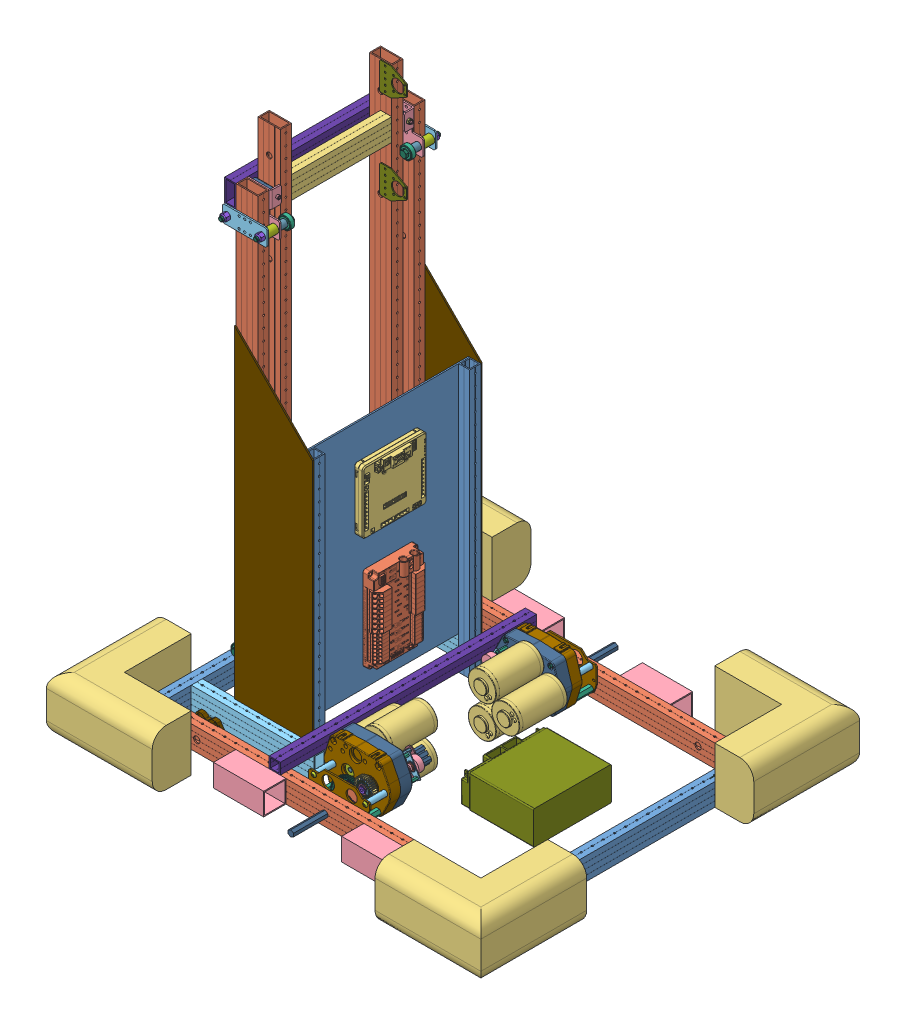
SolidWorks assembly Test Robot 3, configuration Default. Lengths in mm. (continued)
Components (placement in the parent): (continued)
- Test Base 3-1: Test Base 3 [Default] at (-213.2986 -131.6714 217.4582) size (990.6 641.86 863.6) (continued)
  - 3 CIM Ball Shifter with WCD Output-2: 3 CIM Ball Shifter with WCD Output [Default] at (640.2827 400.7203 338.8075) x (0 1 0) z (0 0 -1) size (169.11 183.68 312.65) (continued)
    - 217-3288-001 Rev3-1: 217-3288-001 Rev3 [Default] at (0 0 0.0889) x (0.055929 -0.998435 0) z (0 0 1) size (99.51 99.53 98.3) (continued)
      - 217-2428-007 Rev1-4: 217-2428-007 Rev1 [Default] at (0 -6.275 26.9494) x (-0.766153 0.629782 0.128005) z (-0.605376 -0.640389 -0.472676) size (6.35 6.35 6.35)
      - 217-2428-007 Rev1-5: 217-2428-007 Rev1 [Default] at (-7.809 4.5085 14.2494) x (-0.049287 -0.826019 -0.561483) z (0.929754 -0.24331 0.276329) size (6.35 6.35 6.35)
      - 217-2428-007 Rev1-6: 217-2428-007 Rev1 [Default] at (0 -9.017 14.2494) x (0.739997 0.370326 -0.561483) z (-0.254164 0.926846 0.276329) size (6.35 6.35 6.35)
    - 217-3210-001 Rev1_30t-1: 217-3210-001 Rev1_30t [Default] at (0 53.4162 30.0736) x (-0.966828 0.255427 0) z (0 0 1) size (41.01 41.12 12.65)
    - 217-2711-002 Rev1_50t-1: 217-2711-002 Rev1_50t [Default] at (0 53.4162 17.4244) x (0.262208 -0.965011 0) z (0 0 1) size (66.7 66.76 12.65)
  - Base Front Rail-2: Base Front Rail [Default] at (1069.5219 360.9185 -429.2377) size (25.4 50.8 152.4)
  - Blue Bumper-3: Blue Bumper [Default] at (180.5219 335.5185 942.3623) size (241.3 127 241.3)
  - Blue Bumper-4: Blue Bumper [Default] at (180.5219 335.5185 78.7623) x (0 0 1) z (-1 0 0) size (241.3 127 241.3)
  - Battery_12V-1: Battery_12V [Default] at (955.2219 397.7318 461.8714) x (0 0 1) z (-1 0 0) size (177.8 76.2 167.13)
  - Superstructure Lower Crossbar-2: Superstructure Lower Crossbar [Default] at (561.5219 399.0185 967.7623) x (0 1 0) z (0 0 -1) size (25.4 25.4 584.2)
  - Base Rear Rail-2: Base Rear Rail [Default] at (1069.5219 360.9185 104.1623) size (25.4 50.8 685.8)
  - 217-3432-STEP-v2-1: 217-3432-STEP-v2 [Default] at (383.7219 362.5822 245.4498) size (69.4 66.32 9.53)
  - 217-3432-STEP-v2-2: 217-3432-STEP-v2 [Default] at (383.7219 362.5822 775.6748) x (-1 0 0) z (0 0 -1) size (69.4 66.32 9.53)
  - Electronics Upright-1: Electronics Upright [Default] at (536.1219 1084.8185 688.3623) x (1 0 0) z (0 -1 0) size (25.4 25.4 609.6)
  - Electronics Upright-2: Electronics Upright [Default] at (536.1219 1084.8185 332.7623) x (1 0 0) z (0 -1 0) size (25.4 25.4 609.6)
- Elevator Moving Stage-1: Elevator Moving Stage [Default] at (-744.0684 626.0553 1293.6415) x (0 0 -1) z (1 0 0) size (355.24 1067.72 119.92)
  - Elevator Fixed Frame-1: Elevator Fixed Frame [Default] at (692.621 1.7594 927.1918) x (1 0 0) z (0 1 0) size (25.4 50.8 1066.8)
  - Elevator Fixed Frame-2: Elevator Fixed Frame [Default] at (438.621 1.7594 927.1918) x (1 0 0) z (0 1 0) size (25.4 50.8 1066.8)
  - Elevator Crossbar-1: Elevator Crossbar [Default] at (1200.621 -252.2406 927.1918) x (0 -1 0) z (-1 0 0) size (25.4 50.8 228.6)
  - am-3844+2x1+Elevator+Assembly+Example-1: am-3844+2x1+Elevator+Assembly+Example [Default] at (298.921 81.9689 954.3698) x (-1 0 0) z (0 0 1) size (82.37 89.82 113.91)
    - Example Single Corner Bearing Assembly-1: Example Single Corner Bearing Assembly [Default] at (-442.3285 289.2703 9.4128) x (0 0 1) z (-1 0 0) size (113.91 89.82 82.37)
      - Large Bearing Block Plate-1: Large Bearing Block Plate [Default] at (-85.6128 70.3392 -35.9285) x (1 0 0) z (0 -1 0) size (101.6 24.99 88.9)
      - Small Bearing Block Plate-1: Small Bearing Block Plate [Default] at (-85.6128 70.3392 -64.5035) x (1 0 0) z (0 -1 0) size (101.6 3.17 38.1)
      - 1614Z Bearing-1: 1614Z Bearing [Default] at (-74.6273 89.3892 -8.941) x (-0.590982 0.806685 0) z (0 0 1) size (28.58 28.58 9.53)
      - 1614Z Bearing-2: 1614Z Bearing [Default] at (5.0017 89.3892 -8.941) x (0.001674 0.999999 0) z (0 0 1) size (28.58 28.58 9.53)
      - AS75-18-64 Aluminum Spacer-1: AS75-18-64 Aluminum Spacer [Default] at (5.0017 89.3892 -35.9285) x (-0.668699 0.743533 0) z (-0.743533 -0.668699 0) size (19.05 25.41 19.05)
      - AS75-18-64 Aluminum Spacer-2: AS75-18-64 Aluminum Spacer [Default] at (-74.6273 89.3892 -61.3285) x (0.536222 0.844077 0) z (0.844077 -0.536222 0) size (19.05 25.41 19.05)
      - 3-8-16 NyLock Nut - Mcm 95615A140_95615A140-1: 3-8-16 NyLock Nut - Mcm 95615A140_95615A140 [Default] at (5.0017 89.3892 -64.5035) x (1 0 0) z (0 1 0) size (14.29 12 16.5)
      - 3-8-16 NyLock Nut - Mcm 95615A140_95615A140-2: 3-8-16 NyLock Nut - Mcm 95615A140_95615A140 [Default] at (-74.6273 89.3892 -64.5035) x (1 0 0) z (0 1 0) size (14.29 12 16.5)
      - am-0602 .250 x .192 x 2.14 Brass Tube-1: am-0602 .250 x .192 x 2.14 Brass Tube [Default] at (-7.6348 38.5892 -20.4599) x (0 0 1) z (-1 0 0) size (6.35 6.35 54.36)
      - 13RS075051 .750 x .260 x 1.00 Spacer-1: 13RS075051 .750 x .260 x 1.00 Spacer [Default] at (-60.2128 38.5892 -20.4599) x (0 -0.722855 0.691) z (0 0.691 0.722855) size (19.05 25.4 19.05)
      - 13RS075051 .750 x .260 x 1.00 Spacer-2: 13RS075051 .750 x .260 x 1.00 Spacer [Default] at (-34.8128 38.5892 -20.4599) x (0 -0.801304 -0.598258) z (0 -0.598258 0.801304) size (19.05 25.4 19.05)
      - 0.25 Flat Washer_Preferred Wide FW 0.25-1: 0.25 Flat Washer_Preferred Wide FW 0.25 [Default] at (-60.2128 38.5892 -20.4599) x (1 0 0) z (0 -0.116572 0.993182) size (1.4 15.88 15.88)
      - 0.25 Flat Washer_Preferred Wide FW 0.25-2: 0.25 Flat Washer_Preferred Wide FW 0.25 [Default] at (-8.0158 38.5892 -20.4599) size (1.4 15.88 15.88)
      - 10-32 Nylock Nut-1: 10-32 Nylock Nut [Default] at (-65.1658 38.5892 -20.4599) x (0 -0.097883 0.995198) z (-1 0 0) size (9.53 11 5.96)
      - SHCS 10-32 x 2.75_HX-SHCS 0.19-32x2.75x0.875-C-1: SHCS 10-32 x 2.75_HX-SHCS 0.19-32x2.75x0.875-C [Default] at (0.3662 38.5892 -20.4599) x (-1 0 0) z (0 0.982583 -0.185827) size (74.68 7.94 7.94)
      - AS62-18-56 Aluminum Spacer-1: AS62-18-56 Aluminum Spacer [Default] at (5.0017 89.3892 -13.7035) x (0.977193 0.212353 0) z (-0.212353 0.977193 0) size (15.88 19.06 15.88)
      - AS62-18-56 Aluminum Spacer-2: AS62-18-56 Aluminum Spacer [Default] at (-74.6273 89.3892 -13.7035) x (1 0 0) z (0 1 0) size (15.88 19.06 15.88)
      - 375-16 x 3 Hex Bolt_HFBOLT 0.375-16x2.5x1-C-1: 375-16 x 3 Hex Bolt_HFBOLT 0.375-16x2.5x1-C [Default] at (-74.6273 89.3892 1.9937) x (0 0 -1) z (1 0 0) size (82.37 16.48 14.28)
      - 375-16 x 3 Hex Bolt_HFBOLT 0.375-16x2.5x1-C-2: 375-16 x 3 Hex Bolt_HFBOLT 0.375-16x2.5x1-C [Default] at (5.0017 89.3892 1.9937) x (0 0 -1) z (-0.5 -0.866025 0) size (82.37 16.48 14.28)
  - am-3844+2x1+Elevator+Assembly+Example-2: am-3844+2x1+Elevator+Assembly+Example [Default] at (832.321 81.9689 900.0138) x (1 0 0) z (0 0 -1) size (82.37 89.82 113.91)
    - Example Single Corner Bearing Assembly-1: Example Single Corner Bearing Assembly [Default] at (-442.3285 289.2703 9.4128) x (0 0 1) z (-1 0 0) size (113.91 89.82 82.37)
      - Large Bearing Block Plate-1: Large Bearing Block Plate [Default] at (-85.6128 70.3392 -35.9285) x (1 0 0) z (0 -1 0) size (101.6 24.99 88.9)
      - Small Bearing Block Plate-1: Small Bearing Block Plate [Default] at (-85.6128 70.3392 -64.5035) x (1 0 0) z (0 -1 0) size (101.6 3.17 38.1)
      - 1614Z Bearing-1: 1614Z Bearing [Default] at (-74.6273 89.3892 -8.941) x (-0.590982 0.806685 0) z (0 0 1) size (28.58 28.58 9.53)
      - 1614Z Bearing-2: 1614Z Bearing [Default] at (5.0017 89.3892 -8.941) x (0.001674 0.999999 0) z (0 0 1) size (28.58 28.58 9.53)
      - AS75-18-64 Aluminum Spacer-1: AS75-18-64 Aluminum Spacer [Default] at (5.0017 89.3892 -35.9285) x (-0.668699 0.743533 0) z (-0.743533 -0.668699 0) size (19.05 25.41 19.05)
      - AS75-18-64 Aluminum Spacer-2: AS75-18-64 Aluminum Spacer [Default] at (-74.6273 89.3892 -61.3285) x (0.536222 0.844077 0) z (0.844077 -0.536222 0) size (19.05 25.41 19.05)
      - 3-8-16 NyLock Nut - Mcm 95615A140_95615A140-1: 3-8-16 NyLock Nut - Mcm 95615A140_95615A140 [Default] at (5.0017 89.3892 -64.5035) x (1 0 0) z (0 1 0) size (14.29 12 16.5)
      - 3-8-16 NyLock Nut - Mcm 95615A140_95615A140-2: 3-8-16 NyLock Nut - Mcm 95615A140_95615A140 [Default] at (-74.6273 89.3892 -64.5035) x (1 0 0) z (0 1 0) size (14.29 12 16.5)
      - am-0602 .250 x .192 x 2.14 Brass Tube-1: am-0602 .250 x .192 x 2.14 Brass Tube [Default] at (-7.6348 38.5892 -20.4599) x (0 0 1) z (-1 0 0) size (6.35 6.35 54.36)
      - 13RS075051 .750 x .260 x 1.00 Spacer-1: 13RS075051 .750 x .260 x 1.00 Spacer [Default] at (-60.2128 38.5892 -20.4599) x (0 -0.722855 0.691) z (0 0.691 0.722855) size (19.05 25.4 19.05)
      - 13RS075051 .750 x .260 x 1.00 Spacer-2: 13RS075051 .750 x .260 x 1.00 Spacer [Default] at (-34.8128 38.5892 -20.4599) x (0 -0.801304 -0.598258) z (0 -0.598258 0.801304) size (19.05 25.4 19.05)
      - 0.25 Flat Washer_Preferred Wide FW 0.25-1: 0.25 Flat Washer_Preferred Wide FW 0.25 [Default] at (-60.2128 38.5892 -20.4599) x (1 0 0) z (0 -0.116572 0.993182) size (1.4 15.88 15.88)
      - 0.25 Flat Washer_Preferred Wide FW 0.25-2: 0.25 Flat Washer_Preferred Wide FW 0.25 [Default] at (-8.0158 38.5892 -20.4599) size (1.4 15.88 15.88)
      - 10-32 Nylock Nut-1: 10-32 Nylock Nut [Default] at (-65.1658 38.5892 -20.4599) x (0 -0.097883 0.995198) z (-1 0 0) size (9.53 11 5.96)
      - SHCS 10-32 x 2.75_HX-SHCS 0.19-32x2.75x0.875-C-1: SHCS 10-32 x 2.75_HX-SHCS 0.19-32x2.75x0.875-C [Default] at (0.3662 38.5892 -20.4599) x (-1 0 0) z (0 0.982583 -0.185827) size (74.68 7.94 7.94)
      - AS62-18-56 Aluminum Spacer-1: AS62-18-56 Aluminum Spacer [Default] at (5.0017 89.3892 -13.7035) x (0.977193 0.212353 0) z (-0.212353 0.977193 0) size (15.88 19.06 15.88)
      - AS62-18-56 Aluminum Spacer-2: AS62-18-56 Aluminum Spacer [Default] at (-74.6273 89.3892 -13.7035) x (1 0 0) z (0 1 0) size (15.88 19.06 15.88)
      - 375-16 x 3 Hex Bolt_HFBOLT 0.375-16x2.5x1-C-1: 375-16 x 3 Hex Bolt_HFBOLT 0.375-16x2.5x1-C [Default] at (-74.6273 89.3892 1.9937) x (0 0 -1) z (1 0 0) size (82.37 16.48 14.28)
      - 375-16 x 3 Hex Bolt_HFBOLT 0.375-16x2.5x1-C-2: 375-16 x 3 Hex Bolt_HFBOLT 0.375-16x2.5x1-C [Default] at (5.0017 89.3892 1.9937) x (0 0 -1) z (-0.5 -0.866025 0) size (82.37 16.48 14.28)
  - VersaFrame Side Bearing Mount-1: VersaFrame Side Bearing Mount [Default] at (677.635 719.3094 968.4668) x (0 -1 0) z (1 0 0) size (63.5 61.91 2.29)
  - Elevator Crossbar-2: Elevator Crossbar [Default] at (-69.379 624.0594 939.8918) x (0 0 -1) z (1 0 0) size (25.4 50.8 228.6)
  - VersaFrame Side Bearing Mount-2: VersaFrame Side Bearing Mount [Default] at (677.635 516.1094 968.4668) x (0 -1 0) z (1 0 0) size (63.5 61.91 2.29)
- Elevator Base Frame-1: Elevator Base Frame [Default] at (917.7191 512.449 119.177) x (0 0 1) z (-1 0 0) size (419.1 1066.8 119.57)
  - Elevator Fixed Frame-1: Elevator Fixed Frame [Default] at (786.6435 8.8982 734.5957) x (1 0 0) z (0 1 0) size (25.4 50.8 1066.8)
  - Elevator Fixed Frame-2: Elevator Fixed Frame [Default] at (431.0435 8.8982 734.5957) x (1 0 0) z (0 1 0) size (25.4 50.8 1066.8)
  - am-3844+2x1+Elevator+Assembly+Example-1: am-3844+2x1+Elevator+Assembly+Example [Default] at (37.3435 1067.0077 761.7737) x (-1 0 0) z (0 0 1) size (82.37 89.82 113.91)
    - Example Single Corner Bearing Assembly-1: Example Single Corner Bearing Assembly [Default] at (-442.3285 289.2703 9.4128) x (0 0 1) z (-1 0 0) size (113.91 89.82 82.37)
      - Large Bearing Block Plate-1: Large Bearing Block Plate [Default] at (-85.6128 70.3392 -35.9285) x (1 0 0) z (0 -1 0) size (101.6 24.99 88.9)
      - Small Bearing Block Plate-1: Small Bearing Block Plate [Default] at (-85.6128 70.3392 -64.5035) x (1 0 0) z (0 -1 0) size (101.6 3.17 38.1)
      - 1614Z Bearing-1: 1614Z Bearing [Default] at (-74.6273 89.3892 -8.941) x (-0.590982 0.806685 0) z (0 0 1) size (28.58 28.58 9.53)
      - 1614Z Bearing-2: 1614Z Bearing [Default] at (5.0017 89.3892 -8.941) x (0.001674 0.999999 0) z (0 0 1) size (28.58 28.58 9.53)
      - AS75-18-64 Aluminum Spacer-1: AS75-18-64 Aluminum Spacer [Default] at (5.0017 89.3892 -35.9285) x (-0.668699 0.743533 0) z (-0.743533 -0.668699 0) size (19.05 25.41 19.05)
      - AS75-18-64 Aluminum Spacer-2: AS75-18-64 Aluminum Spacer [Default] at (-74.6273 89.3892 -61.3285) x (0.536222 0.844077 0) z (0.844077 -0.536222 0) size (19.05 25.41 19.05)
      - 3-8-16 NyLock Nut - Mcm 95615A140_95615A140-1: 3-8-16 NyLock Nut - Mcm 95615A140_95615A140 [Default] at (5.0017 89.3892 -64.5035) x (1 0 0) z (0 1 0) size (14.29 12 16.5)
      - 3-8-16 NyLock Nut - Mcm 95615A140_95615A140-2: 3-8-16 NyLock Nut - Mcm 95615A140_95615A140 [Default] at (-74.6273 89.3892 -64.5035) x (1 0 0) z (0 1 0) size (14.29 12 16.5)
      - am-0602 .250 x .192 x 2.14 Brass Tube-1: am-0602 .250 x .192 x 2.14 Brass Tube [Default] at (-7.6348 38.5892 -20.4599) x (0 0 1) z (-1 0 0) size (6.35 6.35 54.36)
      - 13RS075051 .750 x .260 x 1.00 Spacer-1: 13RS075051 .750 x .260 x 1.00 Spacer [Default] at (-60.2128 38.5892 -20.4599) x (0 -0.722855 0.691) z (0 0.691 0.722855) size (19.05 25.4 19.05)
      - 13RS075051 .750 x .260 x 1.00 Spacer-2: 13RS075051 .750 x .260 x 1.00 Spacer [Default] at (-34.8128 38.5892 -20.4599) x (0 -0.801304 -0.598258) z (0 -0.598258 0.801304) size (19.05 25.4 19.05)
      - 0.25 Flat Washer_Preferred Wide FW 0.25-1: 0.25 Flat Washer_Preferred Wide FW 0.25 [Default] at (-60.2128 38.5892 -20.4599) x (1 0 0) z (0 -0.116572 0.993182) size (1.4 15.88 15.88)
      - 0.25 Flat Washer_Preferred Wide FW 0.25-2: 0.25 Flat Washer_Preferred Wide FW 0.25 [Default] at (-8.0158 38.5892 -20.4599) size (1.4 15.88 15.88)
      - 10-32 Nylock Nut-1: 10-32 Nylock Nut [Default] at (-65.1658 38.5892 -20.4599) x (0 -0.097883 0.995198) z (-1 0 0) size (9.53 11 5.96)
      - SHCS 10-32 x 2.75_HX-SHCS 0.19-32x2.75x0.875-C-1: SHCS 10-32 x 2.75_HX-SHCS 0.19-32x2.75x0.875-C [Default] at (0.3662 38.5892 -20.4599) x (-1 0 0) z (0 0.982583 -0.185827) size (74.68 7.94 7.94)
      - AS62-18-56 Aluminum Spacer-1: AS62-18-56 Aluminum Spacer [Default] at (5.0017 89.3892 -13.7035) x (0.977193 0.212353 0) z (-0.212353 0.977193 0) size (15.88 19.06 15.88)
      - AS62-18-56 Aluminum Spacer-2: AS62-18-56 Aluminum Spacer [Default] at (-74.6273 89.3892 -13.7035) x (1 0 0) z (0 1 0) size (15.88 19.06 15.88)
      - 375-16 x 3 Hex Bolt_HFBOLT 0.375-16x2.5x1-C-1: 375-16 x 3 Hex Bolt_HFBOLT 0.375-16x2.5x1-C [Default] at (-74.6273 89.3892 1.9937) x (0 0 -1) z (1 0 0) size (82.37 16.48 14.28)
      - 375-16 x 3 Hex Bolt_HFBOLT 0.375-16x2.5x1-C-2: 375-16 x 3 Hex Bolt_HFBOLT 0.375-16x2.5x1-C [Default] at (5.0017 89.3892 1.9937) x (0 0 -1) z (-0.5 -0.866025 0) size (82.37 16.48 14.28)
  - am-3844+2x1+Elevator+Assembly+Example-2: am-3844+2x1+Elevator+Assembly+Example [Default] at (1180.3435 1067.0077 710.9737) x (1 0 0) z (0 0 -1) size (82.37 89.82 113.91)
    - Example Single Corner Bearing Assembly-1: Example Single Corner Bearing Assembly [Default] at (-442.3285 289.2703 9.4128) x (0 0 1) z (-1 0 0) size (113.91 89.82 82.37)
      - Large Bearing Block Plate-1: Large Bearing Block Plate [Default] at (-85.6128 70.3392 -35.9285) x (1 0 0) z (0 -1 0) size (101.6 24.99 88.9)
      - Small Bearing Block Plate-1: Small Bearing Block Plate [Default] at (-85.6128 70.3392 -64.5035) x (1 0 0) z (0 -1 0) size (101.6 3.17 38.1)
      - 1614Z Bearing-1: 1614Z Bearing [Default] at (-74.6273 89.3892 -8.941) x (-0.590982 0.806685 0) z (0 0 1) size (28.58 28.58 9.53)
      - 1614Z Bearing-2: 1614Z Bearing [Default] at (5.0017 89.3892 -8.941) x (0.001674 0.999999 0) z (0 0 1) size (28.58 28.58 9.53)
      - AS75-18-64 Aluminum Spacer-1: AS75-18-64 Aluminum Spacer [Default] at (5.0017 89.3892 -35.9285) x (-0.668699 0.743533 0) z (-0.743533 -0.668699 0) size (19.05 25.41 19.05)
      - AS75-18-64 Aluminum Spacer-2: AS75-18-64 Aluminum Spacer [Default] at (-74.6273 89.3892 -61.3285) x (0.536222 0.844077 0) z (0.844077 -0.536222 0) size (19.05 25.41 19.05)
      - 3-8-16 NyLock Nut - Mcm 95615A140_95615A140-1: 3-8-16 NyLock Nut - Mcm 95615A140_95615A140 [Default] at (5.0017 89.3892 -64.5035) x (1 0 0) z (0 1 0) size (14.29 12 16.5)
      - 3-8-16 NyLock Nut - Mcm 95615A140_95615A140-2: 3-8-16 NyLock Nut - Mcm 95615A140_95615A140 [Default] at (-74.6273 89.3892 -64.5035) x (1 0 0) z (0 1 0) size (14.29 12 16.5)
      - am-0602 .250 x .192 x 2.14 Brass Tube-1: am-0602 .250 x .192 x 2.14 Brass Tube [Default] at (-7.6348 38.5892 -20.4599) x (0 0 1) z (-1 0 0) size (6.35 6.35 54.36)
      - 13RS075051 .750 x .260 x 1.00 Spacer-1: 13RS075051 .750 x .260 x 1.00 Spacer [Default] at (-60.2128 38.5892 -20.4599) x (0 -0.722855 0.691) z (0 0.691 0.722855) size (19.05 25.4 19.05)
      - 13RS075051 .750 x .260 x 1.00 Spacer-2: 13RS075051 .750 x .260 x 1.00 Spacer [Default] at (-34.8128 38.5892 -20.4599) x (0 -0.801304 -0.598258) z (0 -0.598258 0.801304) size (19.05 25.4 19.05)
      - 0.25 Flat Washer_Preferred Wide FW 0.25-1: 0.25 Flat Washer_Preferred Wide FW 0.25 [Default] at (-60.2128 38.5892 -20.4599) x (1 0 0) z (0 -0.116572 0.993182) size (1.4 15.88 15.88)
      - 0.25 Flat Washer_Preferred Wide FW 0.25-2: 0.25 Flat Washer_Preferred Wide FW 0.25 [Default] at (-8.0158 38.5892 -20.4599) size (1.4 15.88 15.88)
      - 10-32 Nylock Nut-1: 10-32 Nylock Nut [Default] at (-65.1658 38.5892 -20.4599) x (0 -0.097883 0.995198) z (-1 0 0) size (9.53 11 5.96)
      - SHCS 10-32 x 2.75_HX-SHCS 0.19-32x2.75x0.875-C-1: SHCS 10-32 x 2.75_HX-SHCS 0.19-32x2.75x0.875-C [Default] at (0.3662 38.5892 -20.4599) x (-1 0 0) z (0 0.982583 -0.185827) size (74.68 7.94 7.94)
      - AS62-18-56 Aluminum Spacer-1: AS62-18-56 Aluminum Spacer [Default] at (5.0017 89.3892 -13.7035) x (0.977193 0.212353 0) z (-0.212353 0.977193 0) size (15.88 19.06 15.88)
      - AS62-18-56 Aluminum Spacer-2: AS62-18-56 Aluminum Spacer [Default] at (-74.6273 89.3892 -13.7035) x (1 0 0) z (0 1 0) size (15.88 19.06 15.88)
      - 375-16 x 3 Hex Bolt_HFBOLT 0.375-16x2.5x1-C-1: 375-16 x 3 Hex Bolt_HFBOLT 0.375-16x2.5x1-C [Default] at (-74.6273 89.3892 1.9937) x (0 0 -1) z (1 0 0) size (82.37 16.48 14.28)
      - 375-16 x 3 Hex Bolt_HFBOLT 0.375-16x2.5x1-C-2: 375-16 x 3 Hex Bolt_HFBOLT 0.375-16x2.5x1-C [Default] at (5.0017 89.3892 1.9937) x (0 0 -1) z (-0.5 -0.866025 0) size (82.37 16.48 14.28)
  - Frame Crossbar-1: Frame Crossbar [Default] at (1167.6435 732.7982 772.6957) x (0 0 1) z (-1 0 0) size (25.4 50.8 381)
- Elevator Side Panels-1: Elevator Side Panels [Default] at (157.7234 254.6472 918.5205) size (177.8 736.6 3.17)
- Elevator Side Panels-2: Elevator Side Panels [Default] at (157.7234 254.6472 534.3455) size (177.8 736.6 3.17)
- Electronics Panel-1: Electronics Panel [Default] at (306.9484 280.0472 918.5205) x (0 0 -1) z (1 0 0) size (381 533.4 3.17)
- PowerDistributionPanel-1: PowerDistributionPanel [Default] at (316.8036 414.5094 723.415) x (0 -1 0) z (0 0 1) size (192.68 39.24 124.89)
- roboRIO-1: roboRIO [Default] at (319.7754 665.6573 728.661) x (0 0 -1) z (1 0 0) size (146.27 143.19 36.83)
Mates (geometry in assembly coordinates):
- Coincident1: coincident anti-aligned: plane of Test Base 3-1/Base Side Rail Internal-1 through (360.9234 203.8472 918.5205) normal (0 0 -1); plane of Elevator Base Frame-1/Elevator Fixed Frame-1 through (157.7234 1270.6472 918.5205) normal (0 0 1)
- Coincident2: coincident aligned: plane of Test Base 3-1/Base Side Rail Internal-1 through (360.9234 203.8472 943.9205) normal (0 -1 0); plane of Elevator Base Frame-1/Elevator Fixed Frame-1 through (183.1234 203.8472 905.8205) normal (0 -1 0)
- Distance1: distance = 76.2 mm anti-aligned: plane of Elevator Base Frame-1/Elevator Fixed Frame-1 through (157.7234 1270.6472 893.1205) normal (-1 0 0); plane of Test Base 3-1/Base Rear Rail-1 through (81.5234 203.8472 1070.9205) normal (1 0 0)
- Coincident3: coincident aligned: plane of Elevator Moving Stage-1/Elevator Fixed Frame-1 through (208.5234 1377.1147 613.7205) normal (1 0 0); plane of Elevator Base Frame-1/Elevator Fixed Frame-2 through (208.5234 1270.6472 537.5205) normal (1 0 0)
- Distance2: distance = 25.4 mm anti-aligned: plane of Elevator Moving Stage-1/Elevator Fixed Frame-1 through (208.5234 1377.1147 588.3205) normal (0 0 -1); plane of Elevator Base Frame-1/Elevator Fixed Frame-2 through (157.7234 1270.6472 562.9205) normal (0 0 1)
- Coincident4: coincident anti-aligned: plane of Elevator Base Frame-1/Elevator Fixed Frame-1 through (157.7234 1270.6472 918.5205) normal (0 0 1); plane of Elevator Side Panels-1 through (157.7234 254.6472 918.5205) normal (0 0 -1)
- Coincident5: coincident aligned: plane of Elevator Base Frame-1/Elevator Fixed Frame-1 through (157.7234 1270.6472 893.1205) normal (-1 0 0); plane of Elevator Side Panels-1 through (157.7234 254.6472 921.6955) normal (-1 0 0)
- Coincident7: coincident anti-aligned: plane of Elevator Base Frame-1/Elevator Fixed Frame-2 through (157.7234 1270.6472 537.5205) normal (0 0 -1); plane of Elevator Side Panels-2 through (157.7234 254.6472 537.5205) normal (0 0 1)
- Coincident9: coincident aligned: plane of Elevator Base Frame-1/Elevator Fixed Frame-2 through (157.7234 1270.6472 537.5205) normal (-1 0 0); plane of Elevator Side Panels-2 through (157.7234 254.6472 537.5205) normal (-1 0 0)
- Coincident10: coincident anti-aligned: plane of Test Base 3-1/Base Side Rail Internal-1 through (360.9234 254.6472 943.9205) normal (0 1 0); plane of Elevator Side Panels-1 through (157.7234 254.6472 921.6955) normal (0 -1 0)
- Coincident11: coincident anti-aligned: plane of Test Base 3-1/Base Side Rail Internal-4 through (81.5234 254.6472 512.1205) normal (0 1 0); plane of Elevator Side Panels-2 through (157.7234 254.6472 537.5205) normal (0 -1 0)
- Coincident12: coincident anti-aligned: plane of Test Base 3-1/Electronics Upright-2 through (310.1234 203.8472 537.5205) normal (-1 0 0); plane of Electronics Panel-1 through (310.1234 280.0472 918.5205) normal (1 0 0)
- Coincident13: coincident aligned: plane of Test Base 3-1/Electronics Upright-1 through (322.8234 813.4472 905.8205) normal (0 1 0); plane of Electronics Panel-1 through (310.1234 813.4472 918.5205) normal (0 1 0)
- Coincident14: coincident anti-aligned: plane of Elevator Side Panels-1 through (157.7234 254.6472 918.5205) normal (0 0 -1); plane of Electronics Panel-1 through (310.1234 280.0472 918.5205) normal (0 0 1)
- Coincident15: coincident anti-aligned: plane of Electronics Panel-1 through (310.1234 280.0472 918.5205) normal (1 0 0); plane of PowerDistributionPanel-1 through (310.1234 322.4852 780.819) normal (-1 0 0)
- Coincident16: coincident aligned: plane of Electronics Panel-1 through (310.1234 280.0472 918.5205) normal (1 0 0); plane of roboRIO-1 through (310.1234 593.6906 802.173) normal (1 0 0)
- Distance7: distance = 76.2 mm anti-aligned: plane of roboRIO-1 through (312.3555 737.2472 660.587) normal (0 -1 0); plane of Electronics Panel-1 through (310.1234 813.4472 918.5205) normal (0 1 0)
- Distance8: distance = 92.6647 mm aligned: plane of roboRIO-1 through (312.3555 599.1286 655.5852) normal (0 0 1); plane of Test Base 3-1/Electronics Upright-2 through (310.1234 203.8472 562.9205) normal (0 0 1)
- Coincident17: coincident anti-aligned: plane of Electronics Panel-1 through (310.1234 280.0472 918.5205) normal (1 0 0); plane of PowerDistributionPanel-1 through (310.1234 322.4852 780.819) normal (-1 0 0)
